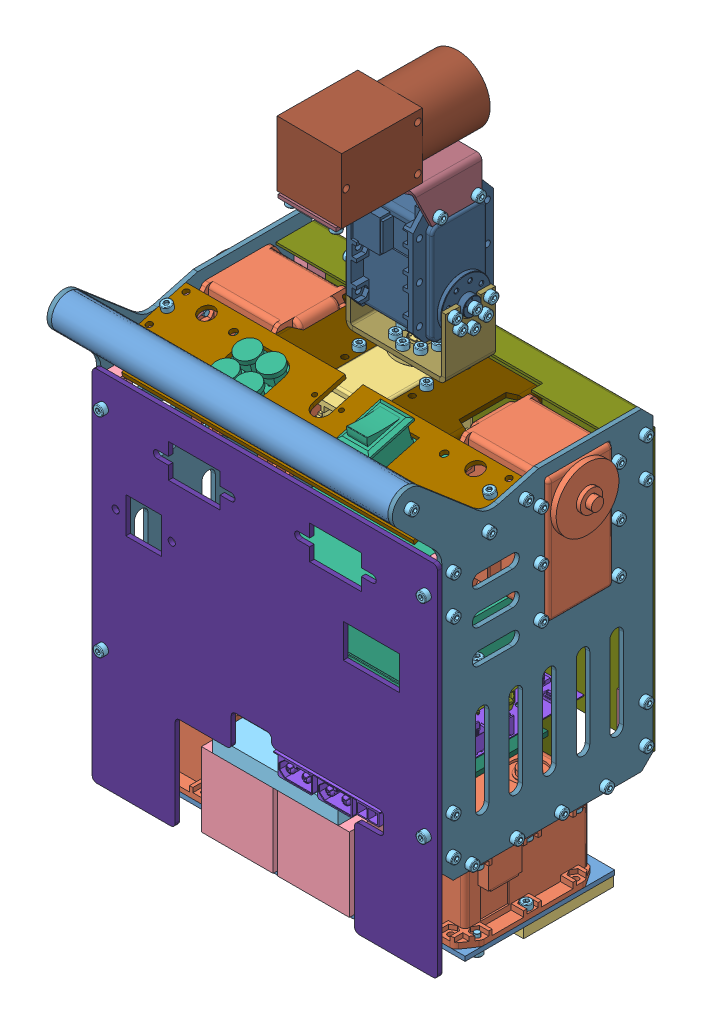
SolidWorks assembly 躯干, configuration 默认. Lengths in mm. (continued)
Mates (geometry in assembly coordinates): (continued)
- 重合144: coincident: plane of assembly; plane of assembly; plane of 机器人-侧板-4 through (91.1339 139.1722 141.05) normal (1 0 0); plane of hexagon socket head cap screws gb-14 through (91.1339 43.9855 136.55) normal (-1 0 0)
- 同心243: concentric: cylinder of assembly; cylinder of assembly; cylinder of 机器人-侧板-4 through (89.1339 43.9855 156.55) axis (1 0 0) radius 1.35; cylinder of hexagon socket head cap screws gb-15 through (85.1339 43.9855 156.55) axis (1 0 0) radius 1.25
- 重合145: coincident: plane of assembly; plane of assembly; plane of 机器人-侧板-4 through (91.1339 139.1722 141.05) normal (1 0 0); plane of hexagon socket head cap screws gb-15 through (91.1339 43.9855 156.55) normal (-1 0 0)
- 同心244: concentric: cylinder of assembly; cylinder of assembly; cylinder of 机器人-侧板-4 through (89.1339 43.9855 176.55) axis (1 0 0) radius 1.35; cylinder of hexagon socket head cap screws gb-16 through (85.1339 43.9855 176.55) axis (1 0 0) radius 1.25
- 重合146: coincident: plane of assembly; plane of assembly; plane of 机器人-侧板-4 through (91.1339 139.1722 141.05) normal (1 0 0); plane of hexagon socket head cap screws gb-16 through (91.1339 43.9855 176.55) normal (-1 0 0)
- 同心245: concentric: cylinder of assembly; cylinder of assembly; cylinder of 机器人-侧板-4 through (91.1349 50.9855 184.95) axis (-1 0 0) radius 1.35; cylinder of hexagon socket head cap screws gb-17 through (85.1339 50.9855 184.95) axis (1 0 0) radius 1.25
- 重合147: coincident: plane of assembly; plane of assembly; plane of 机器人-侧板-4 through (91.1339 139.1722 141.05) normal (1 0 0); plane of hexagon socket head cap screws gb-17 through (91.1339 50.9855 184.95) normal (-1 0 0)
- 同心246: concentric: cylinder of assembly; cylinder of assembly; cylinder of 机器人-侧板-4 through (91.1349 67.9855 184.95) axis (-1 0 0) radius 1.35; cylinder of hexagon socket head cap screws gb-18 through (85.1339 67.9855 184.95) axis (1 0 0) radius 1.25
- 重合148: coincident: plane of assembly; plane of assembly; plane of 机器人-侧板-4 through (91.1339 139.1722 141.05) normal (1 0 0); plane of hexagon socket head cap screws gb-18 through (91.1339 67.9855 184.95) normal (-1 0 0)
- 同心247: concentric: cylinder of assembly; cylinder of assembly; cylinder of 机器人-侧板-4 through (91.1349 160.9855 184.95) axis (-1 0 0) radius 1.35; cylinder of hexagon socket head cap screws gb-19 through (85.1339 160.9855 184.95) axis (1 0 0) radius 1.25
- 重合149: coincident: plane of assembly; plane of assembly; plane of 机器人-侧板-4 through (91.1339 139.1722 141.05) normal (1 0 0); plane of hexagon socket head cap screws gb-19 through (91.1339 160.9855 184.95) normal (-1 0 0)
- 同心248: concentric: cylinder of assembly; cylinder of assembly; cylinder of 机器人-侧板-4 through (91.1349 143.9855 184.95) axis (-1 0 0) radius 1.35; cylinder of hexagon socket head cap screws gb-20 through (85.1339 143.9855 184.95) axis (1 0 0) radius 1.25
- 重合150: coincident: plane of assembly; plane of assembly; plane of 机器人-侧板-4 through (91.1339 139.1722 141.05) normal (1 0 0); plane of hexagon socket head cap screws gb-20 through (91.1339 143.9855 184.95) normal (-1 0 0)
- 同心249: concentric: cylinder of assembly; cylinder of assembly; cylinder of 机器人-侧板-4 through (91.1349 168.5856 168.95) axis (-1 0 0) radius 1.35; cylinder of hexagon socket head cap screws gb-21 through (85.1339 168.5856 168.95) axis (1 0 0) radius 1.25
- 重合151: coincident: plane of assembly; plane of assembly; plane of 机器人-侧板-4 through (91.1339 139.1722 141.05) normal (1 0 0); plane of hexagon socket head cap screws gb-21 through (91.1339 168.5856 168.95) normal (-1 0 0)
- 同心250: concentric: cylinder of assembly; cylinder of assembly; cylinder of 机器人-侧板-4 through (91.1349 172.9855 152.5293) axis (-1 0 0) radius 1.35; cylinder of hexagon socket head cap screws gb-22 through (85.1339 172.9855 152.5293) axis (1 0 0) radius 1.25
- 重合152: coincident: plane of assembly; plane of assembly; plane of 机器人-侧板-4 through (91.1339 139.1722 141.05) normal (1 0 0); plane of hexagon socket head cap screws gb-22 through (91.1339 172.9855 152.5293) normal (-1 0 0)
- 同心251: concentric: cylinder of assembly; cylinder of assembly; cylinder of 机器人-侧板-3 through (-60.8651 170.9855 98.95) axis (-1 0 0) radius 1.35; cylinder of hexagon socket head cap screws gb-23 through (-56.8661 170.9855 98.95) axis (-1 0 0) radius 1.25
- 重合153: coincident: plane of assembly; plane of assembly; plane of 机器人-侧板-3 through (-62.8661 139.1722 141.05) normal (-1 0 0); plane of hexagon socket head cap screws gb-23 through (-62.8661 170.9855 98.95) normal (1 0 0)
- 同心252: concentric: cylinder of assembly; cylinder of assembly; cylinder of 机器人-侧板-3 through (-60.8651 153.9855 98.95) axis (-1 0 0) radius 1.35; cylinder of hexagon socket head cap screws gb-24 through (-56.8661 153.9855 98.95) axis (-1 0 0) radius 1.25
- 重合154: coincident: plane of assembly; plane of assembly; plane of 机器人-侧板-3 through (-62.8661 139.1722 141.05) normal (-1 0 0); plane of hexagon socket head cap screws gb-24 through (-62.8661 153.9855 98.95) normal (1 0 0)
- 同心253: concentric: cylinder of assembly; cylinder of assembly; cylinder of 机器人-侧板-3 through (-60.8651 67.9855 98.95) axis (-1 0 0) radius 1.35; cylinder of hexagon socket head cap screws gb-25 through (-56.8661 67.9855 98.95) axis (-1 0 0) radius 1.25
- 重合155: coincident: plane of assembly; plane of assembly; plane of 机器人-侧板-3 through (-62.8661 139.1722 141.05) normal (-1 0 0); plane of hexagon socket head cap screws gb-25 through (-62.8661 67.9855 98.95) normal (1 0 0)
- 同心254: concentric: cylinder of assembly; cylinder of assembly; cylinder of 机器人-侧板-3 through (-60.8651 50.9855 98.95) axis (-1 0 0) radius 1.35; cylinder of hexagon socket head cap screws gb-26 through (-56.8661 50.9855 98.95) axis (-1 0 0) radius 1.25
- 重合156: coincident: plane of assembly; plane of assembly; plane of 机器人-侧板-3 through (-62.8661 139.1722 141.05) normal (-1 0 0); plane of hexagon socket head cap screws gb-26 through (-62.8661 50.9855 98.95) normal (1 0 0)
- 同心255: concentric: cylinder of assembly; cylinder of assembly; cylinder of 机器人-侧板-3 through (-62.8661 43.9855 116.55) axis (1 0 0) radius 1.35; cylinder of hexagon socket head cap screws gb-27 through (-56.8661 43.9855 116.55) axis (-1 0 0) radius 1.25
- 重合157: coincident: plane of assembly; plane of assembly; plane of 机器人-侧板-3 through (-62.8661 139.1722 141.05) normal (-1 0 0); plane of hexagon socket head cap screws gb-27 through (-62.8661 43.9855 116.55) normal (1 0 0)
- 同心256: concentric: cylinder of assembly; cylinder of assembly; cylinder of 机器人-侧板-3 through (-62.8661 43.9855 136.55) axis (1 0 0) radius 1.35; cylinder of hexagon socket head cap screws gb-28 through (-56.8661 43.9855 136.55) axis (-1 0 0) radius 1.25
- 重合158: coincident: plane of assembly; plane of assembly; plane of 机器人-侧板-3 through (-62.8661 139.1722 141.05) normal (-1 0 0); plane of hexagon socket head cap screws gb-28 through (-62.8661 43.9855 136.55) normal (1 0 0)
- 同心257: concentric: cylinder of assembly; cylinder of assembly; cylinder of 机器人-侧板-3 through (-62.8661 43.9855 156.55) axis (1 0 0) radius 1.35; cylinder of hexagon socket head cap screws gb-29 through (-56.8661 43.9855 156.55) axis (-1 0 0) radius 1.25
- 重合159: coincident: plane of assembly; plane of assembly; plane of 机器人-侧板-3 through (-62.8661 139.1722 141.05) normal (-1 0 0); plane of hexagon socket head cap screws gb-29 through (-62.8661 43.9855 156.55) normal (1 0 0)
- 同心258: concentric: cylinder of assembly; cylinder of assembly; cylinder of 机器人-侧板-3 through (-62.8661 43.9855 176.55) axis (1 0 0) radius 1.35; cylinder of hexagon socket head cap screws gb-30 through (-56.8661 43.9855 176.55) axis (-1 0 0) radius 1.25
- 重合160: coincident: plane of assembly; plane of assembly; plane of 机器人-侧板-3 through (-62.8661 139.1722 141.05) normal (-1 0 0); plane of hexagon socket head cap screws gb-30 through (-62.8661 43.9855 176.55) normal (1 0 0)
- 同心259: concentric: cylinder of assembly; cylinder of assembly; cylinder of 机器人-侧板-3 through (-60.8651 50.9855 184.95) axis (-1 0 0) radius 1.35; cylinder of hexagon socket head cap screws gb-31 through (-56.8661 50.9855 184.95) axis (-1 0 0) radius 1.25
- 重合161: coincident: plane of assembly; plane of assembly; plane of 机器人-侧板-3 through (-62.8661 139.1722 141.05) normal (-1 0 0); plane of hexagon socket head cap screws gb-31 through (-62.8661 50.9855 184.95) normal (1 0 0)
- 同心260: concentric: cylinder of assembly; cylinder of assembly; cylinder of 机器人-侧板-3 through (-60.8651 67.9855 184.95) axis (-1 0 0) radius 1.35; cylinder of hexagon socket head cap screws gb-32 through (-56.8661 67.9855 184.95) axis (-1 0 0) radius 1.25
- 重合162: coincident: plane of assembly; plane of assembly; plane of 机器人-侧板-3 through (-62.8661 139.1722 141.05) normal (-1 0 0); plane of hexagon socket head cap screws gb-32 through (-62.8661 67.9855 184.95) normal (1 0 0)
- 同心261: concentric: cylinder of assembly; cylinder of assembly; cylinder of 机器人-侧板-3 through (-60.8651 143.9855 184.95) axis (-1 0 0) radius 1.35; cylinder of hexagon socket head cap screws gb-33 through (-56.8661 143.9855 184.95) axis (-1 0 0) radius 1.25
- 重合163: coincident: plane of assembly; plane of assembly; plane of 机器人-侧板-3 through (-62.8661 139.1722 141.05) normal (-1 0 0); plane of hexagon socket head cap screws gb-33 through (-62.8661 143.9855 184.95) normal (1 0 0)
- 同心262: concentric: cylinder of assembly; cylinder of assembly; cylinder of 机器人-侧板-3 through (-60.8651 160.9855 184.95) axis (-1 0 0) radius 1.35; cylinder of hexagon socket head cap screws gb-34 through (-56.8661 160.9855 184.95) axis (-1 0 0) radius 1.25
- 重合164: coincident: plane of assembly; plane of assembly; plane of 机器人-侧板-3 through (-62.8661 139.1722 141.05) normal (-1 0 0); plane of hexagon socket head cap screws gb-34 through (-62.8661 160.9855 184.95) normal (1 0 0)
- 同心263: concentric: cylinder of assembly; cylinder of assembly; cylinder of 机器人-侧板-3 through (-60.8651 168.5856 168.95) axis (-1 0 0) radius 1.35; cylinder of hexagon socket head cap screws gb-35 through (-56.8661 168.5856 168.95) axis (-1 0 0) radius 1.25
- 重合165: coincident: plane of assembly; plane of assembly; plane of 机器人-侧板-3 through (-62.8661 139.1722 141.05) normal (-1 0 0); plane of hexagon socket head cap screws gb-35 through (-62.8661 168.5856 168.95) normal (1 0 0)
- 同心264: concentric: cylinder of assembly; cylinder of assembly; cylinder of 机器人-侧板-3 through (-60.8651 172.9855 152.5293) axis (-1 0 0) radius 1.35; cylinder of hexagon socket head cap screws gb-36 through (-56.8661 172.9855 152.5293) axis (-1 0 0) radius 1.25
- 重合166: coincident: plane of assembly; plane of assembly; plane of 机器人-侧板-3 through (-62.8661 139.1722 141.05) normal (-1 0 0); plane of hexagon socket head cap screws gb-36 through (-62.8661 172.9855 152.5293) normal (1 0 0)
- 同心265: concentric: cylinder of assembly; cylinder of assembly; cylinder of 机器人-背板-1 through (-57.8661 176.5811 162.2925) axis (0 -0.965926 -0.258819) radius 1.35; cylinder of hexagon socket head cap screws gb-37 through (-57.8661 170.7856 160.7396) axis (0 0.965926 0.258819) radius 1.25
- 重合167: coincident: plane of assembly; plane of assembly; plane of 机器人-背板-1 through (14.1339 175.6753 165.6733) normal (0 0.965926 0.258819); plane of hexagon socket head cap screws gb-37 through (-57.8661 176.5811 162.2925) normal (0 -0.965926 -0.258819)
- 同心266: concentric: cylinder of assembly; cylinder of assembly; cylinder of 机器人-背板-1 through (86.1339 176.5811 162.2925) axis (0 -0.965926 -0.258819) radius 1.35; cylinder of hexagon socket head cap screws gb-38 through (86.1339 170.7856 160.7396) axis (0 0.965926 0.258819) radius 1.25
- 重合168: coincident: plane of assembly; plane of assembly; plane of 机器人-背板-1 through (14.1339 175.6753 165.6733) normal (0 0.965926 0.258819); plane of hexagon socket head cap screws gb-38 through (86.1339 176.5811 162.2925) normal (0 -0.965926 -0.258819)
- 同心268: concentric: cylinder of assembly; cylinder of assembly; cylinder of 机器人-后盖-2 through (-57.8661 59.4855 188.949) axis (0 0 1) radius 1.6; cylinder of hexagon socket head cap screws gb-41 through (-57.8661 59.4855 184.95) axis (0 0 1) radius 1.25
- 重合170: coincident: plane of assembly; plane of assembly; plane of 机器人-后盖-2 through (14.1339 100.9855 190.95) normal (0 0 1); plane of hexagon socket head cap screws gb-41 through (-57.8661 59.4855 190.95) normal (0 0 -1)
- 同心269: concentric: cylinder of assembly; cylinder of assembly; cylinder of 机器人-后盖-2 through (86.1339 59.4855 188.949) axis (0 0 1) radius 1.6; cylinder of hexagon socket head cap screws gb-42 through (86.1339 59.4855 184.95) axis (0 0 1) radius 1.25
- 重合171: coincident: plane of assembly; plane of assembly; plane of 机器人-后盖-2 through (14.1339 100.9855 190.95) normal (0 0 1); plane of hexagon socket head cap screws gb-42 through (86.1339 59.4855 190.95) normal (0 0 -1)
- 同心270: concentric: cylinder of assembly; cylinder of assembly; cylinder of 机器人-后盖-2 through (86.1339 152.4855 188.949) axis (0 0 1) radius 1.6; cylinder of hexagon socket head cap screws gb-43 through (86.1339 152.4855 184.95) axis (0 0 1) radius 1.25
- 重合172: coincident: plane of assembly; plane of assembly; plane of 机器人-后盖-2 through (14.1339 100.9855 190.95) normal (0 0 1); plane of hexagon socket head cap screws gb-43 through (86.1339 152.4855 190.95) normal (0 0 -1)
- 同心271: concentric: cylinder of assembly; cylinder of assembly; cylinder of 机器人-后盖-2 through (-57.8661 152.4855 188.949) axis (0 0 1) radius 1.6; cylinder of hexagon socket head cap screws gb-44 through (-57.8661 152.4855 184.95) axis (0 0 1) radius 1.25
- 重合173: coincident: plane of assembly; plane of assembly; plane of 机器人-后盖-2 through (14.1339 100.9855 190.95) normal (0 0 1); plane of hexagon socket head cap screws gb-44 through (-57.8661 152.4855 190.95) normal (0 0 -1)
- 同心272: concentric: cylinder of assembly; cylinder of assembly; cylinder of 机器人-侧板-3 through (-62.8661 166.8855 111.25) axis (1 0 0) radius 1.35; cylinder of hexagon socket head cap screws gb-45 through (-56.8661 166.8855 111.25) axis (-1 0 0) radius 1.25
- 重合174: coincident: plane of assembly; plane of assembly; plane of 机器人-侧板-3 through (-62.8661 139.1722 141.05) normal (-1 0 0); plane of hexagon socket head cap screws gb-45 through (-62.8661 166.8855 111.25) normal (1 0 0)
- 同心273: concentric: cylinder of assembly; cylinder of assembly; cylinder of 机器人-侧板-3 through (-62.8661 144.8855 111.25) axis (1 0 0) radius 1.35; cylinder of hexagon socket head cap screws gb-46 through (-56.8661 144.8855 111.25) axis (-1 0 0) radius 1.25
- 重合175: coincident: plane of assembly; plane of assembly; plane of 机器人-侧板-3 through (-62.8661 139.1722 141.05) normal (-1 0 0); plane of hexagon socket head cap screws gb-46 through (-62.8661 144.8855 111.25) normal (1 0 0)
- 同心274: concentric: cylinder of assembly; cylinder of assembly; cylinder of 机器人-侧板-3 through (-62.8661 144.8855 145.85) axis (1 0 0) radius 1.35; cylinder of hexagon socket head cap screws gb-47 through (-56.8661 144.8855 145.85) axis (-1 0 0) radius 1.25
- 重合176: coincident: plane of assembly; plane of assembly; plane of 机器人-侧板-3 through (-62.8661 139.1722 141.05) normal (-1 0 0); plane of hexagon socket head cap screws gb-47 through (-62.8661 144.8855 145.85) normal (1 0 0)
- 同心275: concentric: cylinder of assembly; cylinder of assembly; cylinder of 机器人-侧板-3 through (-62.8661 122.8855 111.25) axis (1 0 0) radius 1.35; cylinder of hexagon socket head cap screws gb-48 through (-56.8661 122.8855 111.25) axis (-1 0 0) radius 1.25
- 重合177: coincident: plane of assembly; plane of assembly; plane of 机器人-侧板-3 through (-62.8661 139.1722 141.05) normal (-1 0 0); plane of hexagon socket head cap screws gb-48 through (-62.8661 122.8855 111.25) normal (1 0 0)
- 同心276: concentric: cylinder of assembly; cylinder of assembly; cylinder of 机器人-侧板-3 through (-62.8661 122.8855 145.85) axis (1 0 0) radius 1.35; cylinder of hexagon socket head cap screws gb-49 through (-56.8661 122.8855 145.85) axis (-1 0 0) radius 1.25
- 重合178: coincident: plane of assembly; plane of assembly; plane of 机器人-侧板-3 through (-62.8661 139.1722 141.05) normal (-1 0 0); plane of hexagon socket head cap screws gb-49 through (-62.8661 122.8855 145.85) normal (1 0 0)
- 同心277: concentric: cylinder of assembly; cylinder of assembly; cylinder of 机器人-侧板-3 through (-62.8661 166.8855 145.85) axis (1 0 0) radius 1.35; cylinder of hexagon socket head cap screws gb-50 through (-56.8661 166.8855 145.85) axis (-1 0 0) radius 1.25
- 重合179: coincident: plane of assembly; plane of assembly; plane of 机器人-侧板-3 through (-62.8661 139.1722 141.05) normal (-1 0 0); plane of hexagon socket head cap screws gb-50 through (-62.8661 166.8855 145.85) normal (1 0 0)
- 同心278: concentric: cylinder of assembly; cylinder of assembly; cylinder of 脑袋-1/机器人-摄像头固定件-1 through (-1.1995 240.1809 112.7223) axis (-0.999965 0 -0.008321) radius 1.35; cylinder of hexagon socket head cap screws gb-51 through (3.3004 240.1809 112.7598) axis (-0.999965 0 -0.008321) radius 1.25
- 重合180: coincident: plane of assembly; plane of assembly; plane of 脑袋-1/机器人-摄像头固定件-1 through (-2.6786 268.6559 110.2099) normal (-0.999965 0 -0.008321); plane of hexagon socket head cap screws gb-51 through (-2.6994 240.1809 112.7099) normal (0.999965 0 0.008321)
- 同心279: concentric: cylinder of assembly; cylinder of assembly; cylinder of 脑袋-1/机器人-摄像头固定件-1 through (-1.3409 240.1809 129.7218) axis (-0.999965 0 -0.008321) radius 1.35; cylinder of hexagon socket head cap screws gb-52 through (3.1589 240.1809 129.7592) axis (-0.999965 0 -0.008321) radius 1.25
- 重合181: coincident: plane of assembly; plane of assembly; plane of 脑袋-1/机器人-摄像头固定件-1 through (-2.6786 268.6559 110.2099) normal (-0.999965 0 -0.008321); plane of hexagon socket head cap screws gb-52 through (-2.8409 240.1809 129.7093) normal (0.999965 0 0.008321)
- 同心280: concentric: cylinder of assembly; cylinder of assembly; cylinder of 脑袋-1/机器人-摄像头固定件-1 through (28.9375 240.1809 112.9731) axis (0.999965 0 0.008321) radius 1.35; cylinder of hexagon socket head cap screws gb-53 through (24.4377 240.1809 112.9357) axis (0.999965 0 0.008321) radius 1.25
- 重合182: coincident: plane of assembly; plane of assembly; plane of 脑袋-1/机器人-摄像头固定件-1 through (30.4583 268.6559 110.4857) normal (0.999965 0 0.008321); plane of hexagon socket head cap screws gb-53 through (30.4375 240.1809 112.9856) normal (-0.999965 0 -0.008321)
- 同心281: concentric: cylinder of assembly; cylinder of assembly; cylinder of 脑袋-1/机器人-摄像头固定件-1 through (28.7961 240.1809 129.9725) axis (0.999965 0 0.008321) radius 1.35; cylinder of hexagon socket head cap screws gb-54 through (24.2962 240.1809 129.9351) axis (0.999965 0 0.008321) radius 1.25
- 重合183: coincident: plane of assembly; plane of assembly; plane of 脑袋-1/机器人-摄像头固定件-1 through (30.4583 268.6559 110.4857) normal (0.999965 0 0.008321); plane of hexagon socket head cap screws gb-54 through (30.296 240.1809 129.985) normal (-0.999965 0 -0.008321)
- 同心282: concentric: cylinder of assembly; cylinder of assembly; cylinder of 机器人-侧板-4 through (89.1339 166.8855 145.85) axis (1 0 0) radius 1.35; cylinder of hexagon socket head cap screws gb-55 through (85.1339 166.8855 145.85) axis (1 0 0) radius 1.25
- 重合184: coincident: plane of assembly; plane of assembly; plane of 机器人-侧板-4 through (91.1339 139.1722 141.05) normal (1 0 0); plane of hexagon socket head cap screws gb-55 through (91.1339 166.8855 145.85) normal (-1 0 0)
- 同心283: concentric: cylinder of assembly; cylinder of assembly; cylinder of 机器人-侧板-4 through (89.1339 144.8855 145.85) axis (1 0 0) radius 1.35; cylinder of hexagon socket head cap screws gb-56 through (85.1339 144.8855 145.85) axis (1 0 0) radius 1.25
- 重合185: coincident: plane of assembly; plane of assembly; plane of 机器人-侧板-4 through (91.1339 139.1722 141.05) normal (1 0 0); plane of hexagon socket head cap screws gb-56 through (91.1339 144.8855 145.85) normal (-1 0 0)
- 同心284: concentric: cylinder of assembly; cylinder of assembly; cylinder of 机器人-侧板-4 through (89.1339 122.8855 145.85) axis (1 0 0) radius 1.35; cylinder of hexagon socket head cap screws gb-57 through (85.1339 122.8855 145.85) axis (1 0 0) radius 1.25
- 重合186: coincident: plane of assembly; plane of assembly; plane of 机器人-侧板-4 through (91.1339 139.1722 141.05) normal (1 0 0); plane of hexagon socket head cap screws gb-57 through (91.1339 122.8855 145.85) normal (-1 0 0)
- 同心285: concentric: cylinder of assembly; cylinder of assembly; cylinder of 机器人-侧板-4 through (89.1339 166.8855 111.25) axis (1 0 0) radius 1.35; cylinder of hexagon socket head cap screws gb-58 through (85.1339 166.8855 111.25) axis (1 0 0) radius 1.25
- 重合187: coincident: plane of assembly; plane of assembly; plane of 机器人-侧板-4 through (91.1339 139.1722 141.05) normal (1 0 0); plane of hexagon socket head cap screws gb-58 through (91.1339 166.8855 111.25) normal (-1 0 0)
- 同心286: concentric: cylinder of assembly; cylinder of assembly; cylinder of 机器人-侧板-4 through (89.1339 144.8855 111.25) axis (1 0 0) radius 1.35; cylinder of hexagon socket head cap screws gb-59 through (85.1339 144.8855 111.25) axis (1 0 0) radius 1.25
- 重合188: coincident: plane of assembly; plane of assembly; plane of 机器人-侧板-4 through (91.1339 139.1722 141.05) normal (1 0 0); plane of hexagon socket head cap screws gb-59 through (91.1339 144.8855 111.25) normal (-1 0 0)
- 同心287: concentric: cylinder of assembly; cylinder of assembly; cylinder of 机器人-侧板-4 through (89.1339 122.8855 111.25) axis (1 0 0) radius 1.35; cylinder of hexagon socket head cap screws gb-60 through (85.1339 122.8855 111.25) axis (1 0 0) radius 1.25
- 重合189: coincident: plane of assembly; plane of assembly; plane of 机器人-侧板-4 through (91.1339 139.1722 141.05) normal (1 0 0); plane of hexagon socket head cap screws gb-60 through (91.1339 122.8855 111.25) normal (-1 0 0)
- 同心289: concentric: cylinder of assembly; cylinder of assembly; cylinder of 脑袋-1/机器人-脖子-1 through (36.4119 204.3809 129.5359) axis (-0.999965 0 -0.008321) radius 1.1; cylinder of hexagon socket head cap screws gb-62 through (30.4121 204.3809 129.486) axis (0.999965 0 0.008321) radius 1.25
- 重合191: coincident: plane of assembly; plane of assembly; plane of 脑袋-1/机器人-脖子-1 through (36.4785 204.3809 121.5362) normal (0.999965 0 0.008321); plane of hexagon socket head cap screws gb-62 through (36.4119 204.3809 129.5359) normal (-0.999965 0 -0.008321)
- 同心290: concentric: cylinder of assembly; cylinder of assembly; cylinder of 脑袋-1/机器人-脖子-1 through (36.4314 198.724 127.1928) axis (-0.999965 0 -0.008321) radius 1.1; cylinder of hexagon socket head cap screws gb-63 through (30.4316 198.724 127.1429) axis (0.999965 0 0.008321) radius 1.25
- 重合192: coincident: plane of assembly; plane of assembly; plane of 脑袋-1/机器人-脖子-1 through (36.4785 204.3809 121.5362) normal (0.999965 0 0.008321); plane of hexagon socket head cap screws gb-63 through (36.4314 198.724 127.1928) normal (-0.999965 0 -0.008321)
- 同心291: concentric: cylinder of assembly; cylinder of assembly; cylinder of 脑袋-1/机器人-脖子-1 through (36.4785 196.3809 121.5362) axis (-0.999965 0 -0.008321) radius 1.1; cylinder of hexagon socket head cap screws gb-64 through (30.4787 196.3809 121.4862) axis (0.999965 0 0.008321) radius 1.25
- 重合193: coincident: plane of assembly; plane of assembly; plane of 脑袋-1/机器人-脖子-1 through (36.4785 204.3809 121.5362) normal (0.999965 0 0.008321); plane of hexagon socket head cap screws gb-64 through (36.4785 196.3809 121.5362) normal (-0.999965 0 -0.008321)
- 同心292: concentric: cylinder of assembly; cylinder of assembly; cylinder of 脑袋-1/机器人-脖子-1 through (36.5256 198.724 115.8795) axis (-0.999965 0 -0.008321) radius 1.1; cylinder of hexagon socket head cap screws gb-65 through (30.5258 198.724 115.8296) axis (0.999965 0 0.008321) radius 1.25
- 重合194: coincident: plane of assembly; plane of assembly; plane of 脑袋-1/机器人-脖子-1 through (36.4785 204.3809 121.5362) normal (0.999965 0 0.008321); plane of hexagon socket head cap screws gb-65 through (36.5256 198.724 115.8795) normal (-0.999965 0 -0.008321)
- 同心293: concentric: cylinder of assembly; cylinder of assembly; cylinder of 脑袋-1/机器人-脖子-1 through (36.5451 204.3809 113.5364) axis (-0.999965 0 -0.008321) radius 1.1; cylinder of hexagon socket head cap screws gb-66 through (30.5453 204.3809 113.4865) axis (0.999965 0 0.008321) radius 1.25
- 重合195: coincident: plane of assembly; plane of assembly; plane of 脑袋-1/机器人-脖子-1 through (36.4785 204.3809 121.5362) normal (0.999965 0 0.008321); plane of hexagon socket head cap screws gb-66 through (36.5451 204.3809 113.5364) normal (-0.999965 0 -0.008321)
- 同心298: concentric: cylinder of assembly; cylinder of assembly; cylinder of 脑袋-1/机器人-脖子-1 through (-8.1987 204.3809 113.1641) axis (0.999965 0 0.008321) radius 1.1; cylinder of hexagon socket head cap screws gb-71 through (-2.1989 204.3809 113.214) axis (-0.999965 0 -0.008321) radius 1.25
- 重合200: coincident: plane of assembly; plane of assembly; plane of 脑袋-1/机器人-脖子-1 through (-8.2653 114.3809 121.1638) normal (-0.999965 0 -0.008321); plane of hexagon socket head cap screws gb-71 through (-8.1987 204.3809 113.1641) normal (0.999965 0 0.008321)
- 同心299: concentric: cylinder of assembly; cylinder of assembly; cylinder of 脑袋-1/机器人-脖子-1 through (-8.2182 198.724 115.5072) axis (0.999965 0 0.008321) radius 1.1; cylinder of hexagon socket head cap screws gb-72 through (-2.2184 198.724 115.5571) axis (-0.999965 0 -0.008321) radius 1.25
- 重合201: coincident: plane of assembly; plane of assembly; plane of 脑袋-1/机器人-脖子-1 through (-8.2653 114.3809 121.1638) normal (-0.999965 0 -0.008321); plane of hexagon socket head cap screws gb-72 through (-8.2182 198.724 115.5072) normal (0.999965 0 0.008321)
- 同心300: concentric: cylinder of assembly; cylinder of assembly; cylinder of 脑袋-1/机器人-脖子-1 through (-8.2653 196.3809 121.1638) axis (0.999965 0 0.008321) radius 1.1; cylinder of hexagon socket head cap screws gb-73 through (-2.2655 196.3809 121.2138) axis (-0.999965 0 -0.008321) radius 1.25
- 重合202: coincident: plane of assembly; plane of assembly; plane of 脑袋-1/机器人-脖子-1 through (-8.2653 114.3809 121.1638) normal (-0.999965 0 -0.008321); plane of hexagon socket head cap screws gb-73 through (-8.2653 196.3809 121.1638) normal (0.999965 0 0.008321)
- 同心301: concentric: cylinder of assembly; cylinder of assembly; cylinder of 脑袋-1/机器人-脖子-1 through (-8.3124 198.724 126.8205) axis (0.999965 0 0.008321) radius 1.1; cylinder of hexagon socket head cap screws gb-74 through (-2.3126 198.724 126.8704) axis (-0.999965 0 -0.008321) radius 1.25
- 重合203: coincident: plane of assembly; plane of assembly; plane of 脑袋-1/机器人-脖子-1 through (-8.2653 114.3809 121.1638) normal (-0.999965 0 -0.008321); plane of hexagon socket head cap screws gb-74 through (-8.3124 198.724 126.8205) normal (0.999965 0 0.008321)
- 同心302: concentric: cylinder of assembly; cylinder of assembly; cylinder of 脑袋-1/机器人-脖子-1 through (-8.3319 204.3809 129.1636) axis (0.999965 0 0.008321) radius 1.1; cylinder of hexagon socket head cap screws gb-75 through (-2.3321 204.3809 129.2135) axis (-0.999965 0 -0.008321) radius 1.25
- 重合204: coincident: plane of assembly; plane of assembly; plane of 脑袋-1/机器人-脖子-1 through (-8.2653 114.3809 121.1638) normal (-0.999965 0 -0.008321); plane of hexagon socket head cap screws gb-75 through (-8.3319 204.3809 129.1636) normal (0.999965 0 0.008321)
- 同心304: concentric: cylinder of assembly; cylinder of assembly; cylinder of MX64-1 through (86.3339 38.4855 168.55) axis (0 1 0) radius 1.35; cylinder of hexagon socket head cap screws gb-78 through (86.3339 44.4855 168.55) axis (0 -1 0) radius 1.25
- 重合206: coincident: plane of assembly; plane of assembly; plane of MX64-1 through (83.3629 38.4855 171.1321) normal (0 -1 0); plane of hexagon socket head cap screws gb-78 through (86.3339 38.4855 168.55) normal (0 1 0)
- 同心305: concentric: cylinder of assembly; cylinder of assembly; cylinder of MX64-1 through (86.3339 38.4855 146.55) axis (0 1 0) radius 1.35; cylinder of hexagon socket head cap screws gb-79 through (86.3339 44.4855 146.55) axis (0 -1 0) radius 1.25
- 重合207: coincident: plane of assembly; plane of assembly; plane of MX64-1 through (83.3629 38.4855 149.1321) normal (0 -1 0); plane of hexagon socket head cap screws gb-79 through (86.3339 38.4855 146.55) normal (0 1 0)
- 同心306: concentric: cylinder of assembly; cylinder of assembly; cylinder of MX64-1 through (86.3339 38.4855 124.55) axis (0 1 0) radius 1.35; cylinder of hexagon socket head cap screws gb-80 through (86.3339 44.4855 124.55) axis (0 -1 0) radius 1.25
- 重合208: coincident: plane of assembly; plane of assembly; plane of MX64-1 through (83.3629 38.4855 127.1321) normal (0 -1 0); plane of hexagon socket head cap screws gb-80 through (86.3339 38.4855 124.55) normal (0 1 0)
- 同心307: concentric: cylinder of assembly; cylinder of assembly; cylinder of MX64-2 through (-58.0661 38.4855 124.55) axis (0 1 0) radius 1.35; cylinder of hexagon socket head cap screws gb-81 through (-58.0661 44.4855 124.55) axis (0 -1 0) radius 1.25
- 重合209: coincident: plane of assembly; plane of assembly; plane of MX64-2 through (-60.9792 38.4855 127.1321) normal (0 -1 0); plane of hexagon socket head cap screws gb-81 through (-58.0661 38.4855 124.55) normal (0 1 0)
- 同心308: concentric: cylinder of assembly; cylinder of assembly; cylinder of MX64-2 through (-58.0661 38.4855 146.55) axis (0 1 0) radius 1.35; cylinder of hexagon socket head cap screws gb-82 through (-58.0661 44.4855 146.55) axis (0 -1 0) radius 1.25
- 重合210: coincident: plane of assembly; plane of assembly; plane of MX64-2 through (-60.9792 38.4855 149.1321) normal (0 -1 0); plane of hexagon socket head cap screws gb-82 through (-58.0661 38.4855 146.55) normal (0 1 0)
- 同心309: concentric: cylinder of assembly; cylinder of assembly; cylinder of MX64-2 through (-58.0661 38.4855 168.55) axis (0 1 0) radius 1.35; cylinder of hexagon socket head cap screws gb-83 through (-58.0661 44.4855 168.55) axis (0 -1 0) radius 1.25
- 重合211: coincident: plane of assembly; plane of assembly; plane of MX64-2 through (-60.9792 38.4855 171.1321) normal (0 -1 0); plane of hexagon socket head cap screws gb-83 through (-58.0661 38.4855 168.55) normal (0 1 0)
- 同心310: concentric: cylinder of assembly; cylinder of assembly; cylinder of MX64-2 through (-58.0661 6.9855 124.55) axis (0 1 0) radius 1.35; cylinder of hexagon socket head cap screws gb-84 through (-58.0661 3.4855 124.55) axis (0 1 0) radius 1.25
- 重合212: coincident: plane of assembly; plane of assembly; plane of MX64-2 through (-60.9792 9.4855 127.1321) normal (0 1 0); plane of hexagon socket head cap screws gb-84 through (-58.0661 9.4855 124.55) normal (0 -1 0)
- 同心311: concentric: cylinder of assembly; cylinder of assembly; cylinder of MX64-2 through (-58.0661 6.9855 146.55) axis (0 1 0) radius 1.35; cylinder of hexagon socket head cap screws gb-85 through (-58.0661 3.4855 146.55) axis (0 1 0) radius 1.25
- 重合213: coincident: plane of assembly; plane of assembly; plane of MX64-2 through (-60.9792 9.4855 149.1321) normal (0 1 0); plane of hexagon socket head cap screws gb-85 through (-58.0661 9.4855 146.55) normal (0 -1 0)
- 同心312: concentric: cylinder of assembly; cylinder of assembly; cylinder of 机器人-下腰骨-1 through (-58.0661 6.9855 168.55) axis (0 -1 0) radius 1.35; cylinder of hexagon socket head cap screws gb-86 through (-58.0661 10.9855 168.55) axis (0 -1 0) radius 1.25
- 重合214: coincident: plane of assembly; plane of assembly; plane of 机器人-下腰骨-1 through (14.1339 4.9855 143.3) normal (0 -1 0); plane of hexagon socket head cap screws gb-86 through (-58.0661 4.9855 168.55) normal (0 1 0)
- 同心313: concentric: cylinder of assembly; cylinder of assembly; cylinder of 机器人-下腰骨-1 through (-23.4661 6.9855 168.55) axis (0 -1 0) radius 1.35; cylinder of hexagon socket head cap screws gb-87 through (-23.4661 10.9855 168.55) axis (0 -1 0) radius 1.25
- 重合215: coincident: plane of assembly; plane of assembly; plane of 机器人-下腰骨-1 through (14.1339 4.9855 143.3) normal (0 -1 0); plane of hexagon socket head cap screws gb-87 through (-23.4661 4.9855 168.55) normal (0 1 0)
- 同心315: concentric: cylinder of assembly; cylinder of assembly; cylinder of MX64-1 through (86.3339 6.9855 146.55) axis (0 1 0) radius 1.35; cylinder of hexagon socket head cap screws gb-89 through (86.3339 3.4855 146.55) axis (0 1 0) radius 1.25
- 重合217: coincident: plane of assembly; plane of assembly; plane of MX64-1 through (83.3629 9.4855 149.1321) normal (0 1 0); plane of hexagon socket head cap screws gb-89 through (86.3339 9.4855 146.55) normal (0 -1 0)
- 同心3161: concentric: cylinder of assembly; cylinder of assembly; cylinder of MX64-1 through (86.3339 6.9855 168.55) axis (0 1 0) radius 1.35; cylinder of hexagon socket head cap screws gb-90 through (86.3339 109.1114 168.55) axis (0 1 0) radius 1.25
- 同心317: concentric: cylinder of assembly; cylinder of assembly; cylinder of 机器人-下腰骨-1 through (86.3339 6.9855 168.55) axis (0 -1 0) radius 1.35; cylinder of hexagon socket head cap screws gb-91 through (86.3339 10.9855 168.55) axis (0 -1 0) radius 1.25
- 重合218: coincident: plane of assembly; plane of assembly; plane of 机器人-下腰骨-1 through (14.1339 4.9855 143.3) normal (0 -1 0); plane of hexagon socket head cap screws gb-91 through (86.3339 4.9855 168.55) normal (0 1 0)
- 同心318: concentric: cylinder of assembly; cylinder of assembly; cylinder of MX64-2 through (-23.4661 6.9855 124.55) axis (0 1 0) radius 1.35; cylinder of hexagon socket head cap screws gb-92 through (-23.4661 3.4855 124.55) axis (0 1 0) radius 1.25
- 重合219: coincident: plane of assembly; plane of assembly; plane of MX64-2 through (-26.4371 9.4855 127.1321) normal (0 1 0); plane of hexagon socket head cap screws gb-92 through (-23.4661 9.4855 124.55) normal (0 -1 0)
- 同心319: concentric: cylinder of assembly; cylinder of assembly; cylinder of MX64-2 through (-23.4661 6.9855 146.55) axis (0 1 0) radius 1.35; cylinder of hexagon socket head cap screws gb-93 through (-23.4661 3.4855 146.55) axis (0 1 0) radius 1.25
- 重合220: coincident: plane of assembly; plane of assembly; plane of MX64-2 through (-26.4371 9.4855 149.1321) normal (0 1 0); plane of hexagon socket head cap screws gb-93 through (-23.4661 9.4855 146.55) normal (0 -1 0)
- 同心320: concentric: cylinder of assembly; cylinder of assembly; cylinder of MX64-1 through (51.7339 6.9855 124.55) axis (0 1 0) radius 1.35; cylinder of hexagon socket head cap screws gb-94 through (51.7339 3.4855 124.55) axis (0 1 0) radius 1.25
- 重合221: coincident: plane of assembly; plane of assembly; plane of MX64-1 through (48.8208 9.4855 127.1321) normal (0 1 0); plane of hexagon socket head cap screws gb-94 through (51.7339 9.4855 124.55) normal (0 -1 0)
- 同心321: concentric: cylinder of assembly; cylinder of assembly; cylinder of MX64-1 through (51.7339 6.9855 146.55) axis (0 1 0) radius 1.35; cylinder of hexagon socket head cap screws gb-95 through (51.7339 3.4855 146.55) axis (0 1 0) radius 1.25
- 重合222: coincident: plane of assembly; plane of assembly; plane of MX64-1 through (48.8208 9.4855 149.1321) normal (0 1 0); plane of hexagon socket head cap screws gb-95 through (51.7339 9.4855 146.55) normal (0 -1 0)
- 同心322: concentric: cylinder of assembly; cylinder of assembly; cylinder of 机器人-肩骨-2 through (55.1339 166.8855 111.25) axis (-1 0 0) radius 1.35; cylinder of hexagon socket head cap screws gb-96 through (59.1339 166.8855 111.25) axis (-1 0 0) radius 1.25
- 重合223: coincident: plane of assembly; plane of assembly; plane of 机器人-肩骨-2 through (53.1339 182.5355 128.55) normal (-1 0 0); plane of hexagon socket head cap screws gb-96 through (53.1339 166.8855 111.25) normal (1 0 0)
- 同心323: concentric: cylinder of assembly; cylinder of assembly; cylinder of 机器人-肩骨-2 through (29.1612 175.2582 116.85) axis (0 -1 0) radius 1.35; cylinder of hexagon socket head cap screws gb-97 through (29.1612 169.2582 116.85) axis (0 1 0) radius 1.25
- 重合224: coincident: plane of assembly; plane of assembly; plane of 机器人-肩骨-2 through (45.1112 175.2582 128.55) normal (0 1 0); plane of hexagon socket head cap screws gb-97 through (29.1612 175.2582 116.85) normal (0 -1 0)
- 同心324: concentric: cylinder of assembly; cylinder of assembly; cylinder of 机器人-肩骨-1 through (-0.8934 175.2582 116.85) axis (0 -1 0) radius 1.35; cylinder of hexagon socket head cap screws gb-98 through (-0.8934 169.2582 116.85) axis (0 1 0) radius 1.25
- 重合225: coincident: plane of assembly; plane of assembly; plane of 机器人-肩骨-1 through (-16.8434 175.2582 128.55) normal (0 1 0); plane of hexagon socket head cap screws gb-98 through (-0.8934 175.2582 116.85) normal (0 -1 0)
- 同心325: concentric: cylinder of assembly; cylinder of assembly; cylinder of 机器人-肩骨-1 through (-26.8661 166.8855 111.25) axis (1 0 0) radius 1.35; cylinder of hexagon socket head cap screws gb-99 through (-30.8661 166.8855 111.25) axis (1 0 0) radius 1.25
- 重合226: coincident: plane of assembly; plane of assembly; plane of 机器人-肩骨-1 through (-24.8661 182.5355 128.55) normal (1 0 0); plane of hexagon socket head cap screws gb-99 through (-24.8661 166.8855 111.25) normal (-1 0 0)
- 同心326: concentric: cone of assembly; cylinder of assembly; cone of MX28-3 through (14.1066 181.657 121.35) axis (0 -1 0); cylinder of hexagon socket head cap screws gb-100 through (14.1066 175.8582 121.35) axis (0 1 0) radius 1.25
- 重合227: coincident: plane of MX28-3 through (17.54 181.8582 125.76) normal (0 1 0); plane of hexagon socket head cap screws gb-100 through (14.1066 181.8582 121.35) normal (0 -1 0)
- 同心327: concentric: cone of assembly; cylinder of assembly; cone of 脑袋-1/MX28-2-1 through (37.3297 204.3809 121.5432) axis (0.999965 0 0.008321); cylinder of hexagon socket head cap screws gb-101 through (31.3287 204.3809 121.4933) axis (0.999965 0 0.008321) radius 1.25
- 重合228: coincident: plane of 脑袋-1/MX28-2-1 through (37.2831 205.6013 126.9971) normal (0.999965 0 0.008321); plane of hexagon socket head cap screws gb-101 through (37.3285 204.3809 121.5432) normal (-0.999965 0 -0.008321)
- 同心328: concentric: cylinder of 脑袋-1/MX28-2-1 through (-6.02 204.3809 121.1825) axis (0.999965 0 0.008321) radius 785.3982; cylinder of hexagon socket head cap screws gb-102 through (-0.1202 204.3809 121.2316) axis (-0.999965 0 -0.008321) radius 1.25
- 重合229: coincident: plane of 脑袋-1/MX28-2-1 through (-6.1332 201.2266 122.7693) normal (-0.999965 0 -0.008321); plane of hexagon socket head cap screws gb-102 through (-6.12 204.3809 121.1817) normal (0.999965 0 0.008321)
- 同心329: concentric: cylinder of assembly; cylinder of assembly; cylinder of 机器人-肩骨-1 through (-0.8934 175.2582 133.85) axis (0 -1 0) radius 1.35; cylinder of hexagon socket head cap screws gb-103 through (-0.8934 169.2582 133.85) axis (0 1 0) radius 1.25
- 重合230: coincident: plane of 机器人-肩骨-1 through (-16.8434 175.2582 128.55) normal (0 1 0); plane of hexagon socket head cap screws gb-103 through (-0.8934 175.2582 133.85) normal (0 -1 0)
- 同心330: concentric: cylinder of assembly; cylinder of assembly; cylinder of 机器人-肩骨-1 through (-26.8661 166.8855 145.85) axis (1 0 0) radius 1.35; cylinder of hexagon socket head cap screws gb-104 through (-30.8661 166.8855 145.85) axis (1 0 0) radius 1.25
- 重合231: coincident: plane of 机器人-肩骨-1 through (-24.8661 182.5355 128.55) normal (1 0 0); plane of hexagon socket head cap screws gb-104 through (-24.8661 166.8855 145.85) normal (-1 0 0)
- 同心331: concentric: cylinder of assembly; cylinder of assembly; cylinder of 机器人-肩骨-2 through (55.1339 166.8855 145.85) axis (-1 0 0) radius 1.35; cylinder of hexagon socket head cap screws gb-105 through (59.1339 166.8855 145.85) axis (-1 0 0) radius 1.25
- 重合232: coincident: plane of 机器人-肩骨-2 through (53.1339 182.5355 128.55) normal (-1 0 0); plane of hexagon socket head cap screws gb-105 through (53.1339 166.8855 145.85) normal (1 0 0)
- 同心332: concentric: cylinder of assembly; cylinder of assembly; cylinder of 机器人-肩骨-2 through (29.1612 175.2582 133.85) axis (0 -1 0) radius 1.35; cylinder of hexagon socket head cap screws gb-106 through (29.1612 169.2582 133.85) axis (0 1 0) radius 1.25
- 重合233: coincident: plane of 机器人-肩骨-2 through (45.1112 175.2582 128.55) normal (0 1 0); plane of hexagon socket head cap screws gb-106 through (29.1612 175.2582 133.85) normal (0 -1 0)
- 同心333: concentric: cylinder of assembly; cylinder of assembly; cylinder of 脑袋-1/机器人-脖子-1 through (8.497 179.0082 115.6463) axis (0 1 0) radius 1.1; cylinder of hexagon socket head cap screws gb-107 through (8.497 175.0082 115.6463) axis (0 1 0) radius 1.25
- 重合234: coincident: plane of 脑袋-1/机器人-脖子-1 through (59.105 181.0082 121.7244) normal (0 1 0); plane of hexagon socket head cap screws gb-107 through (8.497 181.0082 115.6463) normal (0 -1 0)
- 同心334: concentric: cylinder of assembly; cylinder of assembly; cylinder of 脑袋-1/机器人-脖子-1 through (6.1069 179.0082 121.2834) axis (0 1 0) radius 1.1; cylinder of hexagon socket head cap screws gb-108 through (6.1069 175.0082 121.2834) axis (0 1 0) radius 1.25
- 重合235: coincident: plane of 脑袋-1/机器人-脖子-1 through (59.105 181.0082 121.7244) normal (0 1 0); plane of hexagon socket head cap screws gb-108 through (6.1069 181.0082 121.2834) normal (0 -1 0)
- 同心335: concentric: cylinder of assembly; cylinder of assembly; cylinder of 脑袋-1/机器人-脖子-1 through (8.4029 179.0082 126.9596) axis (0 1 0) radius 1.1; cylinder of hexagon socket head cap screws gb-109 through (8.4029 175.0082 126.9596) axis (0 1 0) radius 1.25
- 重合236: coincident: plane of 脑袋-1/机器人-脖子-1 through (59.105 181.0082 121.7244) normal (0 1 0); plane of hexagon socket head cap screws gb-109 through (8.4029 181.0082 126.9596) normal (0 -1 0)
- 同心336: concentric: cylinder of assembly; cylinder of assembly; cylinder of 脑袋-1/机器人-脖子-1 through (14.04 179.0082 129.3497) axis (0 1 0) radius 1.1; cylinder of hexagon socket head cap screws gb-110 through (14.04 175.0082 129.3497) axis (0 1 0) radius 1.25
- 重合237: coincident: plane of 脑袋-1/机器人-脖子-1 through (59.105 181.0082 121.7244) normal (0 1 0); plane of hexagon socket head cap screws gb-110 through (14.04 181.0082 129.3497) normal (0 -1 0)
- 同心337: concentric: cylinder of assembly; cylinder of assembly; cylinder of 脑袋-1/机器人-脖子-1 through (19.7162 179.0082 127.0537) axis (0 1 0) radius 1.1; cylinder of hexagon socket head cap screws gb-111 through (19.7162 175.0082 127.0537) axis (0 1 0) radius 1.25
- 重合238: coincident: plane of 脑袋-1/机器人-脖子-1 through (59.105 181.0082 121.7244) normal (0 1 0); plane of hexagon socket head cap screws gb-111 through (19.7162 181.0082 127.0537) normal (0 -1 0)
- 同心338: concentric: cylinder of assembly; cylinder of assembly; cylinder of 脑袋-1/机器人-脖子-1 through (22.1063 179.0082 121.4166) axis (0 1 0) radius 1.1; cylinder of hexagon socket head cap screws gb-112 through (22.1063 175.0082 121.4166) axis (0 1 0) radius 1.25
- 重合239: coincident: plane of 脑袋-1/机器人-脖子-1 through (59.105 181.0082 121.7244) normal (0 1 0); plane of hexagon socket head cap screws gb-112 through (22.1063 181.0082 121.4166) normal (0 -1 0)
- 同心339: concentric: cylinder of assembly; cylinder of assembly; cylinder of 脑袋-1/机器人-脖子-1 through (19.8103 179.0082 115.7404) axis (0 1 0) radius 1.1; cylinder of hexagon socket head cap screws gb-113 through (19.8103 175.0082 115.7404) axis (0 1 0) radius 1.25
- 重合240: coincident: plane of 脑袋-1/机器人-脖子-1 through (59.105 181.0082 121.7244) normal (0 1 0); plane of hexagon socket head cap screws gb-113 through (19.8103 181.0082 115.7404) normal (0 -1 0)
- 同心340: concentric: cylinder of assembly; cylinder of assembly; cylinder of 脑袋-1/机器人-脖子-1 through (14.1732 179.0082 113.3503) axis (0 1 0) radius 1.1; cylinder of hexagon socket head cap screws gb-114 through (14.1732 175.0082 113.3503) axis (0 1 0) radius 1.25
- 重合241: coincident: plane of 脑袋-1/机器人-脖子-1 through (59.105 181.0082 121.7244) normal (0 1 0); plane of hexagon socket head cap screws gb-114 through (14.1732 181.0082 113.3503) normal (0 -1 0)
- 同心341: concentric: cylinder of assembly; cylinder of assembly; cylinder of 机器人-侧板-4 through (91.1339 194.6934 203.5985) axis (-1 0 0) radius 1.6; cylinder of hexagon socket head cap screws gb-115 through (85.1339 194.6934 203.5985) axis (1 0 0) radius 1.25
- 重合242: coincident: plane of 机器人-侧板-4 through (91.1339 139.1722 141.05) normal (1 0 0); plane of hexagon socket head cap screws gb-115 through (91.1339 194.6934 203.5985) normal (-1 0 0)
- 同心342: concentric: cylinder of assembly; cylinder of assembly; cylinder of 机器人-侧板-3 through (-60.8661 194.6934 203.5985) axis (-1 0 0) radius 1.6; cylinder of hexagon socket head cap screws gb-116 through (-56.8661 194.6934 203.5985) axis (-1 0 0) radius 1.25
- 重合243: coincident: plane of 机器人-侧板-3 through (-62.8661 139.1722 141.05) normal (-1 0 0); plane of hexagon socket head cap screws gb-116 through (-62.8661 194.6934 203.5985) normal (1 0 0)
- 同心343: concentric: cylinder of assembly; cylinder of assembly; cylinder of 脑袋-1/机器人-摄像头固定件-1 through (23.6707 252.7249 136.7301) axis (0 1 0) radius 1.6; cylinder of hexagon socket head cap screws gb-117 through (23.6707 258.7249 136.7301) axis (0 -1 0) radius 1.25
- 重合244: coincident: plane of 脑袋-1/机器人-摄像头固定件-1 through (13.8898 252.7249 110.3478) normal (0 -1 0); plane of hexagon socket head cap screws gb-117 through (23.6707 252.7249 136.7301) normal (0 1 0)
- 同心344: concentric: cylinder of assembly; cylinder of assembly; cylinder of 脑袋-1/机器人-摄像头固定件-1 through (3.6713 252.7249 136.5637) axis (0 1 0) radius 1.6; cylinder of hexagon socket head cap screws gb-118 through (3.6713 258.7249 136.5637) axis (0 -1 0) radius 1.25
- 重合245: coincident: plane of 脑袋-1/机器人-摄像头固定件-1 through (13.8898 252.7249 110.3478) normal (0 -1 0); plane of hexagon socket head cap screws gb-118 through (3.6713 252.7249 136.5637) normal (0 1 0)
- 同心345: concentric: cylinder of assembly; cylinder of assembly; cylinder of 脑袋-1/机器人-摄像头固定件-1 through (3.4076 252.7249 168.2626) axis (0 1 0) radius 1.6; cylinder of hexagon socket head cap screws gb-119 through (3.4076 258.7249 168.2626) axis (0 -1 0) radius 1.25
- 重合246: coincident: plane of 脑袋-1/机器人-摄像头固定件-1 through (13.8898 252.7249 110.3478) normal (0 -1 0); plane of hexagon socket head cap screws gb-119 through (3.4076 252.7249 168.2626) normal (0 1 0)
- 同心346: concentric: cylinder of assembly; cylinder of assembly; cylinder of 脑袋-1/机器人-摄像头固定件-1 through (23.4069 252.7249 168.429) axis (0 1 0) radius 1.6; cylinder of hexagon socket head cap screws gb-120 through (23.4069 258.7249 168.429) axis (0 -1 0) radius 1.25
- 重合247: coincident: plane of 脑袋-1/机器人-摄像头固定件-1 through (13.8898 252.7249 110.3478) normal (0 -1 0); plane of hexagon socket head cap screws gb-120 through (23.4069 252.7249 168.429) normal (0 1 0)
- 重合248: coincident: plane of assembly; plane of assembly; plane of 机器人-下腰骨-1 through (-0.8661 6.9855 95.45) normal (0 0 -1); plane of 电池组-1/小电池-1 through (15.3339 43.4855 95.45) normal (0 0 -1)
- 重合249: coincident: plane of assembly; plane of assembly; plane of 机器人-下腰骨-1 through (14.1339 6.9855 143.3) normal (0 1 0); plane of 电池组-1/大电池-1 through (-17.6661 6.9855 109.45) normal (0 -1 0)
- 距离13: distance = 3 mm: plane of 电池组-1/大电池-1 through (-17.6661 39.9855 109.45) normal (-1 0 0); plane of MX64-2 through (-20.6661 11.5927 123.0883) normal (1 0 0)
- 同心3164: concentric: cylinder of assembly; cylinder of assembly; cylinder of 电路-1/Main-1 through (-33.8661 55.9855 117.55) axis (0 -1 0) radius 1.6; cylinder of 机器人-上腰骨-2 through (-33.8661 50.9855 117.55) axis (0 -1 0) radius 1.6
- 同心3165: concentric: cylinder of 电路-1/Main-1 through (-33.8661 55.9855 157.55) axis (0 -1 0) radius 1.6; cylinder of 机器人-上腰骨-2 through (-33.8661 50.9855 157.55) axis (0 -1 0) radius 1.6
- 距离14: distance = 5 mm: plane of 电路-1/Main-1 through (-35.8661 55.9855 165.55) normal (0 -1 0); plane of 机器人-上腰骨-2 through (14.1339 50.9855 149.05) normal (0 1 0)
- 同心3166: concentric: cylinder of assembly; cylinder of assembly; cylinder of 机器人-背板-1 through (-32.8661 177.7458 157.9459) axis (0 -0.965926 -0.258819) radius 1.6; cylinder of Back-1 through (-32.8661 172.5187 156.5453) axis (0 -0.965926 -0.258819) radius 1.6
- 同心3167: concentric: cylinder of assembly; cylinder of assembly; cylinder of 机器人-背板-1 through (-32.8661 172.5694 177.2644) axis (0 -0.965926 -0.258819) radius 1.6; cylinder of Back-1 through (-32.8661 167.3423 175.8638) axis (0 -0.965926 -0.258819) radius 1.6
- 距离15: distance = 5 mm: plane of assembly; plane of assembly; plane of Back-1 through (-35.8661 166.4457 180.7999) normal (0 0.965926 0.258819); plane of 机器人-背板-1 through (14.1339 175.6753 165.6733) normal (0 0.965926 0.258819)
